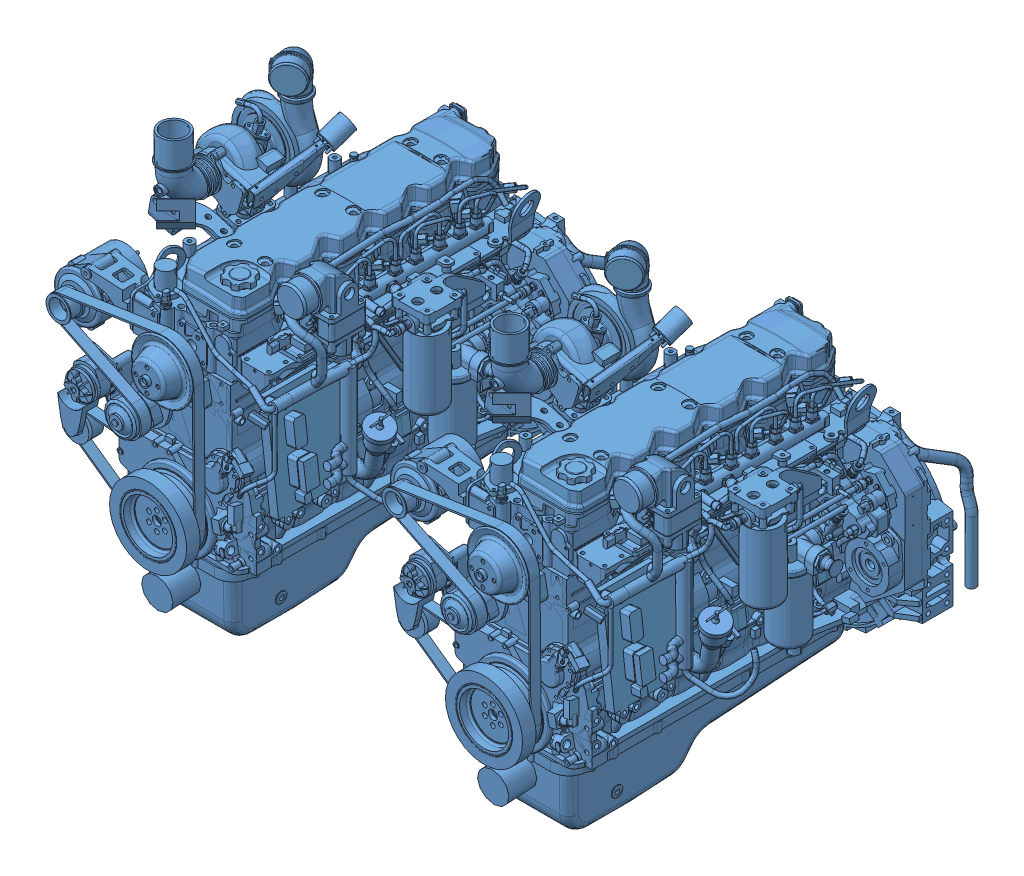
SolidWorks assembly old, configuration Default. Lengths in mm.
Overall size (1640.52 1138.06 1111.89).
2 component instances, 1 part files, 3 mates.
Components (placement in the parent):
- new-1: new [X002623] at origin size (726.12 1138.06 1111.89)
- new-2: new [X002623] at (914.4 0 0) size (726.12 1138.06 1111.89)
Mates (geometry in assembly coordinates):
- Distance1: distance = 914.4 mm: plane of new-2 through (914.4 0 0) normal (1 0 0); plane of assembly
- Coincident2: coincident: plane of new-2 through (914.4 0 0) normal (0 1 0); plane of assembly
- Coincident3: coincident aligned: plane of new-2 through (914.4 0 0) normal (0 0 1); plane of assembly
